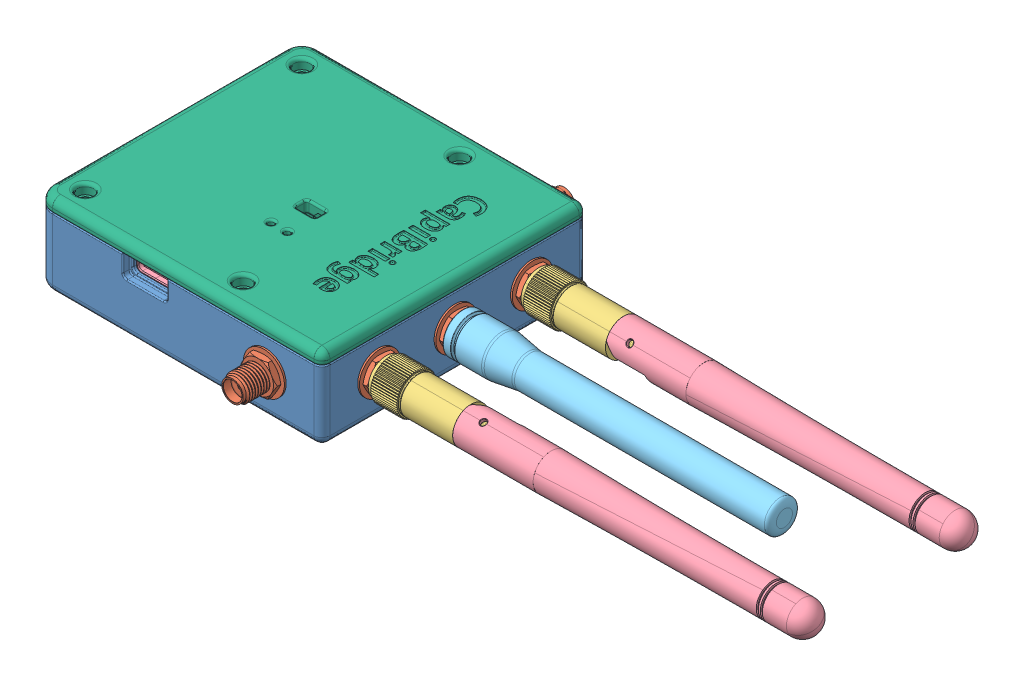
SolidWorks assembly Assem1, configuration Default. Lengths in mm.
Overall size (180.51 20.68 82.51).
87 component instances, 25 part files, 27 mates.
Components (placement in the parent):
- CapiBridge_Case-1: CapiBridge_Case [Default] at (33.8959 31.6338 50.0318) size (71 17.5 66)
- Part1^Assem1-1: Part1^Assem1 [Default] at origin (virtual)
- ESP-NOW_Gateway.step-1: ESP-NOW_Gateway.step [Default] at (0.2771 40.6338 19.0568) x (1 0 0) z (0 1 0) size (44.35 60.13 16.02)
  - C_0603_1608Metric.step-1: C_0603_1608Metric.step [Default] at (27.5987 -37.7 1.63) x (0 1 0) z (0 0 1) size (1.6 0.8 0.8)
    - SOLID.step-1: SOLID.step [Default] at origin size (1.6 0.8 0.8)
  - CP_EIA-3216-18_Kemet-A.step-1: CP_EIA-3216-18_Kemet-A.step [Default] at (19.3987 -47.8 1.63) size (3.2 1.6 1.8)
    - SOLID-0.step-1: SOLID-0.step [Default] at origin size (3.2 1.6 1.8)
  - USB_C_Receptacle_GCT_USB4105-xx-A_16P_TopMnt_Horizontal.step-1: USB_C_Receptacle_GCT_USB4105-xx-A_16P_TopMnt_Horizontal.step [Default] at (25.1087 -57.96 1.63) size (8.94 7.78 4.26)
    - COMPOUND.step-1: COMPOUND.step [Default] at origin size (8.94 7.78 4.26)
  - LED_0603_1608Metric.step-1: LED_0603_1608Metric.step [Default] at (33.4487 -26.2 1.63) size (1.6 0.8 1.1)
    - SOLID-1.step-1: SOLID-1.step [Default] at origin size (1.6 0.8 1.1)
  - YC164-FR-075K6L.step-1: YC164-FR-075K6L.step [Default] at (38.5987 -25.55 1.63) x (1 0 0) z (0 -1 0) size (1.6 0.7 3.2)
    - COMPOUND-2.step-1: COMPOUND-2.step [Default] at origin size (1.6 0.7 3.2)
  - CP_EIA-3528-21_Kemet-B.step-1: CP_EIA-3528-21_Kemet-B.step [Default] at (9.8987 -49.3 1.63) x (0 1 0) z (0 0 1) size (3.5 2.8 2.1)
    - SOLID-3.step-1: SOLID-3.step [Default] at origin size (3.5 2.8 2.1)
  - LED_0603_1608Metric.step-2: LED_0603_1608Metric.step [Default] at (33.4487 -24.65 1.63) size (1.6 0.8 1.1)
    - SOLID-1.step-1: SOLID-1.step [Default] at origin size (1.6 0.8 1.1)
  - ESP32-C3-WROOM-02U-N4.step-1: ESP32-C3-WROOM-02U-N4.step [Default] at (24.0527 -22.934 1.63) size (18 14.3 3.21)
    - COMPOUND-4.step-1: COMPOUND-4.step [Default] at origin size (18 14.3 3.21)
  - SW_SPST_B3U-1000P.step-1: SW_SPST_B3U-1000P.step [Default] at (34.2987 -41.8 1.63) x (0 1 0) z (0 0 1) size (4.8 3.01 1.59)
    - SOLID-5.step-1: SOLID-5.step [Default] at origin size (4.8 3.01 1.59)
  - YC164-FR-075K6L.step-2: YC164-FR-075K6L.step [Default] at (28.4487 -32.8 1.63) x (0 -1 0) z (-1 0 0) size (1.6 0.7 3.2)
    - COMPOUND-2.step-1: COMPOUND-2.step [Default] at origin size (1.6 0.7 3.2)
  - SW_SPST_B3U-1000P.step-2: SW_SPST_B3U-1000P.step [Default] at (38.2987 -41.8 1.63) x (0 -1 0) z (0 0 1) size (4.8 3.01 1.59)
    - SOLID-5.step-1: SOLID-5.step [Default] at origin size (4.8 3.01 1.59)
  - C_0603_1608Metric.step-2: C_0603_1608Metric.step [Default] at (40.1987 -52 1.63) x (0 -1 0) z (0 0 1) size (1.6 0.8 0.8)
    - SOLID.step-1: SOLID.step [Default] at origin size (1.6 0.8 0.8)
  - SOT-363_SC-70-6.step-1: SOT-363_SC-70-6.step [Default] at (34.3487 -47.65 1.63) x (-1 0 0) z (0 0 1) size (2 2 1.05)
    - SOLID-6.step-1: SOLID-6.step [Default] at origin size (2 2 1.05)
  - RA-01H--3DModel-STEP-1.step-1: RA-01H--3DModel-STEP-1.step [Default] at (16.4787 -36.2 1.63) x (1 0 0) z (0 -1 0) size (16 3.4 17)
    - COMPOUND-7.step-1: COMPOUND-7.step [Default] at origin size (16 3.4 17)
  - U.FL_Hirose_U.FL-R-SMT-1_Vertical.step-1: U.FL_Hirose_U.FL-R-SMT-1_Vertical.step [Default] at (8.9987 -24.86 1.63) x (0 1 0) z (0 0 1) size (3.1 3 1.25)
    - SOLID-8.step-1: SOLID-8.step [Default] at origin size (3.1 3 1.25)
  - C_0603_1608Metric.step-3: C_0603_1608Metric.step [Default] at (6.2147 -32.4 1.63) x (0 1 0) z (0 0 1) size (1.6 0.8 0.8)
    - SOLID.step-1: SOLID.step [Default] at origin size (1.6 0.8 0.8)
  - SOT-143.step-1: SOT-143.step [Default] at (25.0851 -50.1648 1.63) size (2.8 2.9 1.2)
    - SOLID-9.step-1: SOLID-9.step [Default] at origin size (2.8 2.9 1.2)
  - C_0603_1608Metric.step-4: C_0603_1608Metric.step [Default] at (2.9664 -9.7709 1.63) x (0 -1 0) z (0 0 1) size (1.6 0.8 0.8)
    - SOLID.step-1: SOLID.step [Default] at origin size (1.6 0.8 0.8)
  - C_0603_1608Metric.step-5: C_0603_1608Metric.step [Default] at (12.5987 -49.8 1.63) x (0 1 0) z (0 0 1) size (1.6 0.8 0.8)
    - SOLID.step-1: SOLID.step [Default] at origin size (1.6 0.8 0.8)
  - ESP32-C3-WROOM-02U-N4.step-2: ESP32-C3-WROOM-02U-N4.step [Default] at (2.9027 -22.908 1.63) size (18 14.3 3.21)
    - COMPOUND-4.step-1: COMPOUND-4.step [Default] at origin size (18 14.3 3.21)
  - SOT-223.step-1: SOT-223.step [Default] at (13.4487 -55.9 1.63) x (-1 0 0) z (0 0 1) size (7 6.5 1.7)
    - SOLID-10.step-1: SOLID-10.step [Default] at origin size (7 6.5 1.7)
  - YC164-FR-075K6L.step-3: YC164-FR-075K6L.step [Default] at (38.5487 -47.2 1.63) x (1 0 0) z (0 -1 0) size (1.6 0.7 3.2)
    - COMPOUND-2.step-1: COMPOUND-2.step [Default] at origin size (1.6 0.7 3.2)
  - C_0603_1608Metric.step-6: C_0603_1608Metric.step [Default] at (29.1987 -37.7 1.63) x (0 1 0) z (0 0 1) size (1.6 0.8 0.8)
    - SOLID.step-1: SOLID.step [Default] at origin size (1.6 0.8 0.8)
  - LED_0603_1608Metric.step-3: LED_0603_1608Metric.step [Default] at (33.4487 -23.05 1.63) size (1.6 0.8 1.1)
    - SOLID-1.step-1: SOLID-1.step [Default] at origin size (1.6 0.8 1.1)
  - Selector Switch - MSS22D18.step-1: Selector Switch - MSS22D18.step [Default] at (36.3987 -31.75 6.88) x (1 0 0) z (0 -1 0) size (9.17 5.82 6.22)
    - SOLID-11.step-1: SOLID-11.step [Default] at origin size (9.17 5.82 6.22)
  - LED_0603_1608Metric.step-4: LED_0603_1608Metric.step [Default] at (28.5487 -48.45 1.63) x (0 1 0) z (0 0 1) size (1.6 0.8 1.1)
    - SOLID-1.step-1: SOLID-1.step [Default] at origin size (1.6 0.8 1.1)
  - SOIC-16_3.9x9.9mm_P1.27mm.step-1: SOIC-16_3.9x9.9mm_P1.27mm.step [Default] at (35.4987 -54.5 1.63) size (6 9.9 1.75)
    - SOLID-12.step-1: SOLID-12.step [Default] at origin size (6 9.9 1.75)
  - C_0603_1608Metric.step-7: C_0603_1608Metric.step [Default] at (24.1807 -9.7222 1.63) x (0 1 0) z (0 0 1) size (1.6 0.8 0.8)
    - SOLID.step-1: SOLID.step [Default] at origin size (1.6 0.8 0.8)
  - LED_0603_1608Metric.step-5: LED_0603_1608Metric.step [Default] at (30.2487 -48.45 1.63) x (0 1 0) z (0 0 1) size (1.6 0.8 1.1)
    - SOLID-1.step-1: SOLID-1.step [Default] at origin size (1.6 0.8 1.1)
  - C_0603_1608Metric.step-8: C_0603_1608Metric.step [Default] at (15.4487 -49 1.63) x (-1 0 0) z (0 0 1) size (1.6 0.8 0.8)
    - SOLID.step-1: SOLID.step [Default] at origin size (1.6 0.8 0.8)
  - LED_0603_1608Metric.step-6: LED_0603_1608Metric.step [Default] at (33.4487 -27.8 1.63) size (1.6 0.8 1.1)
    - SOLID-1.step-1: SOLID-1.step [Default] at origin size (1.6 0.8 1.1)
  - D_SOD-123F.step-1: D_SOD-123F.step [Default] at (19.3987 -50.2 1.63) size (3.5 1.6 1.1)
    - SOLID-13.step-1: SOLID-13.step [Default] at origin size (3.5 1.6 1.1)
  - YC164-FR-075K6L.step-4: YC164-FR-075K6L.step [Default] at (28.3987 -42.4 1.63) x (0 1 0) z (1 0 0) size (1.6 0.7 3.2)
    - COMPOUND-2.step-1: COMPOUND-2.step [Default] at origin size (1.6 0.7 3.2)
  - PinHeader_1x12_P2.54mm_Vertical.step-1: PinHeader_1x12_P2.54mm_Vertical.step [Default] at (3.48 -52.88 -0.05) x (1 0 0) z (0 0 -1) size (2.54 30.48 11.54)
    - SOLID-14.step-1: SOLID-14.step [Default] at origin size (2.54 30.48 11.54)
  - PinHeader_1x12_P2.54mm_Vertical.step-2: PinHeader_1x12_P2.54mm_Vertical.step [Default] at (44.12 -52.9 -0.05) x (1 0 0) z (0 0 -1) size (2.54 30.48 11.54)
    - SOLID-14.step-1: SOLID-14.step [Default] at origin size (2.54 30.48 11.54)
  - PCB.step-1: PCB.step [Default] at origin size (44.35 58.95 1.58)
- 1053072-1-1: 1053072-1 [Default] at (77.6509 38.8838 31.0318) x (0 -1 0) z (1 0 0) size (10.21 10.21 16.97)
- 1053072-1-2: 1053072-1 [Default] at (77.6509 38.8838 50.0318) x (0 -1 0) z (1 0 0) size (10.21 10.21 16.97)
- 1053072-1-3: 1053072-1 [Default] at (77.6509 38.8838 69.0318) x (0 -1 0) z (1 0 0) size (10.21 10.21 16.97)
- 2.4 GHz Antenna.STEP-1: 2.4 GHz Antenna.STEP [Default] at (114.1525 43.2459 32.5323) x (0 0.642694 0.766123) z (-1 0 0) size (10 9.99 107.5)
  - 2.4 GHz Antenna Base.STEP-1: 2.4 GHz Antenna Base.STEP [Default] at (-3.953 -2.3775 34.75) size (10 9.99 28.5)
  - 2.4 GHz Antenna Top.STEP-1: 2.4 GHz Antenna Top.STEP [Default] at (-3.953 -2.3775 1.75) size (9.01 9.28 86.5)
- 2.4 GHz Antenna.STEP-2: 2.4 GHz Antenna.STEP [Default] at (114.1525 34.3011 69.5584) x (0 -0.910184 -0.414204) z (-1 0 0) size (10 9.99 107.5)
  - 2.4 GHz Antenna Base.STEP-1: 2.4 GHz Antenna Base.STEP [Default] at (-3.953 -2.3775 34.75) size (10 9.99 28.5)
  - 2.4 GHz Antenna Top.STEP-1: 2.4 GHz Antenna Top.STEP [Default] at (-3.953 -2.3775 1.75) size (9.01 9.28 86.5)
- 80mm antenna SMA-1: 80mm antenna SMA [Default] at (71.4025 38.8838 50.0318) x (0 -0.641104 0.767454) z (0 0.767454 0.641104) size (10 80.14 10)
- 1053072-1-4: 1053072-1 [Default] at (55.3959 38.8838 8.7768) x (0 1 0) z (0 0 -1) size (10.21 10.21 16.97)
- 1053072-1-5: 1053072-1 [Default] at (55.3959 38.8838 91.2868) x (0 -1 0) z (0 0 1) size (10.21 10.21 16.97)
- CapiBridge_Case_lit-1: CapiBridge_Case_lit [Default] at (33.8959 31.6338 50.0318) size (71 7.48 66)
Mates (geometry in assembly coordinates):
- Parallel3: parallel anti-aligned: plane of CapiBridge_Case-1 through (1.3959 46.6338 20.0318) normal (1 0 0); plane of ESP-NOW_Gateway.step-1/PCB.step-1 through (1.9271 40.6338 76.9568) normal (-1 0 0)
- Coincident2: coincident anti-aligned: plane of CapiBridge_Case-1 through (4.4759 40.6338 23.1068) normal (0 1 0); plane of ESP-NOW_Gateway.step-1/PCB.step-1 through (24.1021 40.6338 50.0318) normal (0 -1 0)
- Concentric5: concentric anti-aligned: cylinder of CapiBridge_Case-1 through (4.4759 40.6338 23.1068) axis (0 -1 0) radius 1.4; cylinder of ESP-NOW_Gateway.step-1/PCB.step-1 through (4.4759 39.8438 23.1068) axis (0 1 0) radius 1.1
- Parallel4: parallel anti-aligned: plane of CapiBridge_Case-1 through (-1.6051 36.2138 32.7032) normal (0 1 0); plane of 1053072-1-1 through (66.2209 36.1406 36.5223) normal (0 -1 0)
- Parallel5: parallel anti-aligned: plane of CapiBridge_Case-1 through (-1.6051 36.2138 51.7032) normal (0 1 0); plane of 1053072-1-2 through (66.2209 36.1406 55.5223) normal (0 -1 0)
- Parallel6: parallel anti-aligned: plane of CapiBridge_Case-1 through (-1.6051 36.2138 70.7032) normal (0 1 0); plane of 1053072-1-3 through (66.2209 36.1406 74.5223) normal (0 -1 0)
- Concentric6: concentric anti-aligned: cylinder of CapiBridge_Case-1 through (-1.6051 38.8838 69.0318) axis (1 0 0) radius 3.15; cylinder of 1053072-1-3 through (78.2224 38.8838 69.0318) axis (-1 0 0) radius 2.3114
- Concentric7: concentric anti-aligned: cylinder of CapiBridge_Case-1 through (-1.6051 38.8838 50.0318) axis (1 0 0) radius 3.15; cylinder of 1053072-1-2 through (78.2224 38.8838 50.0318) axis (-1 0 0) radius 2.3114
- Concentric8: concentric anti-aligned: cylinder of CapiBridge_Case-1 through (-1.6051 38.8838 31.0318) axis (1 0 0) radius 3.15; cylinder of 1053072-1-1 through (78.2224 38.8838 31.0318) axis (-1 0 0) radius 2.3114
- Coincident6: coincident anti-aligned: plane of CapiBridge_Case-1 through (69.3959 46.6338 17.0318) normal (1 0 0); plane of 1053072-1-3 through (69.3959 38.8838 69.0318) normal (-1 0 0)
- Coincident7: coincident anti-aligned: plane of CapiBridge_Case-1 through (69.3959 46.6338 17.0318) normal (1 0 0); plane of 1053072-1-2 through (69.3959 38.8838 50.0318) normal (-1 0 0)
- Coincident8: coincident anti-aligned: plane of CapiBridge_Case-1 through (69.3959 46.6338 17.0318) normal (1 0 0); plane of 1053072-1-1 through (69.3959 38.8838 31.0318) normal (-1 0 0)
- Concentric10: concentric aligned: cylinder of 1053072-1-3 through (78.2224 38.8838 69.0318) axis (-1 0 0) radius 2.3114; cylinder of 2.4 GHz Antenna.STEP-2/2.4 GHz Antenna Base.STEP-1 through (75.4025 38.8838 69.0318) axis (-1 0 0) radius 3.5
- Concentric11: concentric aligned: cylinder of 1053072-1-2 through (78.2224 38.8838 50.0318) axis (-1 0 0) radius 2.3114; cylinder of 80mm antenna SMA-1 through (75.6025 38.8838 50.0318) axis (-1 0 0) radius 0.4
- Coincident9: coincident anti-aligned: plane of 1053072-1-3 through (71.4025 38.8838 69.0318) normal (1 0 0); plane of 2.4 GHz Antenna.STEP-2/2.4 GHz Antenna Base.STEP-1 through (71.4025 38.8838 69.0318) normal (-1 0 0)
- Coincident10: coincident anti-aligned: plane of 1053072-1-2 through (71.4025 38.8838 50.0318) normal (1 0 0); plane of 80mm antenna SMA-1 through (71.4025 38.8838 50.0318) normal (-1 0 0)
- Parallel7: parallel anti-aligned: plane of CapiBridge_Case-1 through (33.8959 36.2138 17.0318) normal (0 1 0); plane of 1053072-1-5 through (49.9054 36.1406 79.8568) normal (0 -1 0)
- Concentric12: concentric anti-aligned: cylinder of CapiBridge_Case-1 through (55.3959 38.8838 17.0318) axis (0 0 1) radius 3.15; cylinder of 1053072-1-5 through (55.3959 38.8838 91.8583) axis (0 0 -1) radius 2.3114
- Coincident12: coincident anti-aligned: plane of CapiBridge_Case-1 through (-1.6041 46.6338 83.0318) normal (0 0 1); plane of 1053072-1-5 through (55.3959 38.8838 83.0318) normal (0 0 -1)
- Parallel8: parallel aligned: plane of CapiBridge_Case-1 through (33.8959 36.2138 17.0318) normal (0 1 0); plane of 1053072-1-4 through (49.9054 41.627 20.2068) normal (0 1 0)
- Concentric13: concentric aligned: cylinder of CapiBridge_Case-1 through (55.3959 38.8838 17.0318) axis (0 0 1) radius 3.15; cylinder of 1053072-1-4 through (55.3959 38.8838 8.2053) axis (0 0 1) radius 2.3114
- Coincident14: coincident anti-aligned: plane of CapiBridge_Case-1 through (-1.6041 46.6338 17.0318) normal (0 0 -1); plane of 1053072-1-4 through (55.3959 38.8838 17.0318) normal (0 0 1)
- Concentric14: concentric aligned: cylinder of 1053072-1-1 through (78.2224 38.8838 31.0318) axis (-1 0 0) radius 2.3114; cylinder of 2.4 GHz Antenna.STEP-1/2.4 GHz Antenna Base.STEP-1 through (75.4025 38.8838 31.0318) axis (-1 0 0) radius 3.5
- Coincident15: coincident anti-aligned: plane of 1053072-1-1 through (71.4025 38.8838 31.0318) normal (1 0 0); plane of 2.4 GHz Antenna.STEP-1/2.4 GHz Antenna Base.STEP-1 through (71.4025 38.8838 31.0318) normal (-1 0 0)
- Coincident16: coincident aligned: plane of CapiBridge_Case-1 through (-1.6041 46.6338 83.0318) normal (0 0 1); plane of CapiBridge_Case_lit-1 through (-1.6041 46.6338 83.0318) normal (0 0 1)
- Coincident17: coincident aligned: plane of CapiBridge_Case-1 through (-1.6041 46.6338 17.0318) normal (-1 0 0); plane of CapiBridge_Case_lit-1 through (-1.6041 46.6338 17.0318) normal (-1 0 0)
- Coincident18: coincident anti-aligned: plane of CapiBridge_Case-1 through (33.8959 46.6338 50.0318) normal (0 1 0); plane of CapiBridge_Case_lit-1 through (-10.4485 46.6338 17.0318) normal (0 -1 0)
